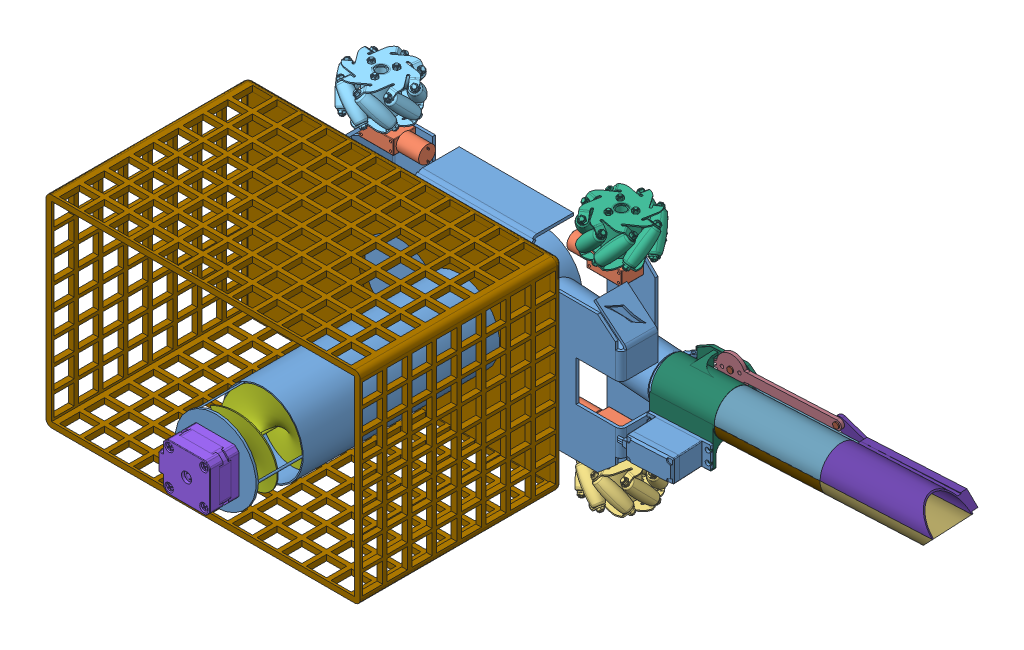
SolidWorks assembly tennis_car4, configuration 默认. Lengths in mm.
Overall size (577.55 226.09 334.13).
29 component instances, 19 part files, 66 mates.
Components (placement in the parent):
- car_main_body-1: car_main_body [默认] at (-145.051 -370.0736 71.4729) x (0 1 0) z (0 0 1) size (155.3 282.12 292.07)
- DC-1: DC [默认] at (85.5314 -436.576 -92.4792) x (-1 0 0) z (0 -1 0) size (53.09 20 29.75)
- Mecanum_wheel_RF-1: Mecanum_wheel_RF [默认] at (115.9795 -500.576 -23.0536) x (0 1 0) z (-0.527874 0 -0.849323) size (37 59.47 59.47)
- DC-2: DC [默认] at (-98.7631 -436.5721 -92.4792) x (1 0 0) z (0 -1 0) size (53.09 20 29.75)
- Mecanum_wheel_RB2-1: Mecanum_wheel_RB2 [默认] at (-98.0143 -496.5968 -67.0588) x (0 -1 0) z (-0.547075 0 -0.837084) size (37 61.04 61.04)
- DC-3: DC [默认] at (-98.7631 -344.5751 -92.4792) x (1 0 0) z (0 1 0) size (53.09 20 29.75)
- Mecanum_wheel_LB2-1: Mecanum_wheel_LB2 [默认] at (-99.6676 -280.5751 -22.7664) x (0 -1 0) z (0.13721 0 -0.990542) size (37 59.47 59.47)
- DC-4: DC [默认] at (85.5314 -344.5712 -92.4792) x (-1 0 0) z (0 1 0) size (53.09 20 29.75)
- Mecanum_wheel_LF2-1: Mecanum_wheel_LF2 [默认] at (125.629 -307.5959 -108.7375) x (0 -1 0) z (-0.82588 0 0.563846) size (37 61.04 61.04)
- spiral_tube-1: spiral_tube [默认] at (4.7184 -390.5736 -116.766) x (0.909362 0.416006 0) z (0 0 1) size (68 68 282.11)
- Stepper Motor3-1: Stepper Motor3 [默认] at (4.7184 -390.5736 198.234) x (0 1 0) z (-1 0 0) size (42 43 47.1)
- box2-1: box2 [默认] at (-48.4877 -300.5736 41.234) x (1 0 0) z (0 -1 0) size (280 180 180)
- part8-8-3: part8-8 [Default] at (159.2089 -414.9542 -121.0328) x (0.049403 0 0.998779) z (0.822654 -0.567084 -0.040691) size (30 17.5 17.5)
- Part6-6-17: Part6-6 [Default] at (266.8876 -408.5259 -124.3565) x (0.382581 -0.923728 -0.018924) z (-0.9226 -0.383049 0.045635) size (5 8 5)
- Part1-2-3: Part1-2 [Default] at (267.0852 -408.5259 -120.3614) x (0.926104 0.374476 -0.045808) z (-0.049403 0 -0.998779) size (119.31 46.68 44)
- Part6-6-18: Part6-6 [Default] at (266.9977 -377.0736 -124.3619) x (-0.382581 0.923728 0.018924) z (0.9226 0.383049 -0.045635) size (5 8 5)
- Part6-6-19: Part6-6 [Default] at (177.1076 -377.0736 -119.9157) x (-0.026872 -0.999638 0.001329) z (-0.998417 0.026905 0.049385) size (5 8 5)
- part5-5-3: part5-5 [Default] at (177.4534 -377.0736 -112.9243) x (-0.049403 0 -0.998779) z (-0.990234 -0.130526 0.04898) size (3 27.84 107.77)
- Part6-6-20: Part6-6 [Default] at (177.5028 -404.0736 -111.9255) x (-0.118763 -0.992905 0.005874) z (0.991693 -0.118909 -0.049052) size (5 8 5)
- Part2-2-3: Part2-2 [Default] at (197.7547 -385.3338 -115.4303) x (0.998779 0.000271 -0.049403) z (0.049403 0 0.998779) size (97 19 41)
- Part3-3-3: Part3-3 [Default] at (139.6032 -390.5736 -117.0594) x (0 -1 0) z (0.049403 0 0.998779) size (57.15 60.42 44.03)
- Part6-6-21: Part6-6 [Default] at (197.483 -385.3338 -120.9235) x (0.382581 -0.923728 -0.018924) z (-0.9226 -0.383049 0.045635) size (5 8 5)
- Part6-6-22: Part6-6 [Default] at (287.3731 -385.3094 -125.3698) x (0.382581 -0.923728 -0.018924) z (-0.9226 -0.383049 0.045635) size (5 8 5)
- Part6-6-23: Part6-6 [Default] at (287.2619 -400.2875 -125.3643) x (0.223935 -0.974541 -0.011077) z (-0.973351 -0.224209 0.048145) size (5 8 5)
- Part6-6-24: Part6-6 [Default] at (197.483 -395.8134 -120.9235) x (0.382581 -0.923728 -0.018924) z (-0.9226 -0.383049 0.045635) size (5 8 5)
- part4-4-3: part4-4 [Default] at (177.3052 -404.0736 -115.9206) x (0.049403 0 0.998779) z (-0.997556 0.049471 0.049342) size (3 29.07 108.54)
- Part1-1-3: Part1-1 [Default] at (267.0471 -377.0736 -123.3632) x (0.926153 -0.374355 -0.04581) z (0.049403 0 0.998779) size (117.54 46.76 44)
- Part2-1-3: Part2-1 [Default] at (287.5336 -400.2875 -119.871) x (-0.997544 0.049712 0.049342) z (0.049403 0 0.998779) size (97 23.44 41)
- 舵机-1: 舵机 [默认] at (171.737 -414.9542 -72.1921) x (-0.998779 0 0.049403) z (0 -1 0) size (56.95 44.55 19.71)
Mates (geometry in assembly coordinates):
- 同心1: concentric aligned: cylinder of car_main_body-1 through (4.7184 -390.5736 171.234) axis (0 0 -1) radius 36; cylinder of spiral_tube-1 through (4.7184 -390.5736 165.234) axis (0 0 -1) radius 1
- 重合13: coincident anti-aligned: plane of car_main_body-1 through (4.7184 -390.5736 -116.766) normal (0 0 1); plane of spiral_tube-1 through (4.7184 -390.5736 -116.766) normal (0 0 -1)
- 同心2: concentric aligned: cylinder of car_main_body-1 through (4.7184 -390.5736 171.234) axis (0 0 1) radius 11; cylinder of Stepper Motor3-1 through (4.7184 -390.5736 155.234) axis (0 0 1) radius 2.5
- 同心3: concentric aligned: circle of car_main_body-1; cone of Stepper Motor3-1 through (20.2184 -375.0736 173.234) axis (0 0 1)
- 重合16: coincident anti-aligned: plane of car_main_body-1 through (4.7184 -390.5736 173.234) normal (0 0 1); plane of Stepper Motor3-1 through (4.7184 -390.5736 173.234) normal (0 0 -1)
- 重合17: coincident anti-aligned: plane of car_main_body-1 through (4.7184 -390.5736 -48.766) normal (0 0 1); plane of box2-1 through (-188.4877 -480.5736 -48.766) normal (0 0 -1)
- 重合18: coincident aligned: plane of car_main_body-1 through (-145.051 -390.5736 71.4729) normal (0 -1 0); plane of box2-1 through (-48.4877 -390.5736 41.234) normal (0 -1 0)
- 同心35: concentric anti-aligned: cylinder of DC-1 through (100.5314 -477.576 -92.4792) axis (0 1 0) radius 4; cylinder of Mecanum_wheel_RF-1 through (100.5314 -470.576 -92.4792) axis (0 -1 0) radius 4
- 重合35: coincident anti-aligned: plane of DC-1 through (100.5314 -470.576 -92.4792) normal (0 -1 0); plane of Mecanum_wheel_RF-1 through (100.5314 -470.576 -92.4792) normal (0 1 0)
- 重合36: coincident: plane of DC-1 through (110.5314 -436.576 -102.4792) normal (0 0 -1); plane of car_main_body-1 through (100.4806 -390.5736 -102.4792) normal (0 0 1)
- 重合37: coincident: plane of car_main_body-1 through (-145.051 -461.576 71.4729) normal (0 -1 0); plane of DC-1 through (85.5314 -461.576 -92.4792) normal (0 -1 0)
- 重合38: coincident: line of car_main_body-1 through (110.5314 -461.576 -104.9792) axis (0 0 1); plane of DC-1 through (110.5314 -461.576 -107.4792) normal (1 0 0)
- 重合39: coincident: plane of car_main_body-1 through (-91.0439 -390.5736 -102.4792) normal (0 0 1); plane of DC-2 through (-123.7631 -436.5721 -102.4792) normal (0 0 -1)
- 重合40: coincident: plane of car_main_body-1 through (-123.6589 -461.5721 -103.9928) normal (0 -1 0); plane of DC-2 through (-98.7631 -461.5721 -92.4792) normal (0 -1 0)
- 重合41: coincident: line of car_main_body-1 through (-123.7631 -445.1021 -102.4792) axis (0 -1 0); plane of DC-2 through (-123.7631 -461.5721 -77.4792) normal (-1 0 0)
- 同心37: concentric anti-aligned: cylinder of DC-3 through (-113.7631 -303.5751 -92.4792) axis (0 -1 0) radius 4; cylinder of Mecanum_wheel_LB2-1 through (-113.7631 -310.5751 -92.4792) axis (0 1 0) radius 4
- 重合42: coincident anti-aligned: plane of DC-3 through (-113.7631 -310.5751 -92.4792) normal (0 1 0); plane of Mecanum_wheel_LB2-1 through (-113.7631 -310.5751 -92.4792) normal (0 -1 0)
- 重合43: coincident: plane of car_main_body-1 through (-91.0439 -390.5736 -102.4792) normal (0 0 1); plane of DC-3 through (-123.7631 -344.5751 -102.4792) normal (0 0 -1)
- 重合44: coincident: plane of car_main_body-1 through (-125.6782 -319.5751 -101.5862) normal (0 1 0); plane of DC-3 through (-98.7631 -319.5751 -92.4792) normal (0 1 0)
- 重合45: coincident: line of car_main_body-1 through (-123.7631 -319.5751 -102.4792) axis (0 -1 0); plane of DC-3 through (-123.7631 -319.5751 -107.4792) normal (-1 0 0)
- 重合47: coincident: plane of car_main_body-1 through (100.4806 -390.5736 -102.4792) normal (0 0 1); plane of DC-4 through (110.5314 -344.5712 -102.4792) normal (0 0 -1)
- 重合48: coincident: plane of car_main_body-1 through (-145.051 -319.5712 71.4729) normal (0 1 0); plane of DC-4 through (85.5314 -319.5712 -92.4792) normal (0 1 0)
- 重合49: coincident: line of car_main_body-1 through (110.5314 -319.5712 -102.4792) axis (0 0 -1); plane of DC-4 through (110.5314 -319.5712 -77.4792) normal (1 0 0)
- GearMate2: gear = 13 : 24 mm: cylinder of part8-8-3 through (159.7029 -414.9542 -111.045) axis (-0.049403 0 -0.998779) radius 5.249; cylinder of part4-4-3 through (177.4534 -404.0736 -112.9243) axis (-0.049403 0 -0.998779) radius 12.0927
- 重合20: coincident aligned: plane of Part3-3-3 through (139.6032 -390.5736 -117.0594) normal (-0.049403 0 -0.998779); plane of part8-8-3 through (159.3571 -414.9542 -118.0365) normal (-0.049403 0 -0.998779)
- 同心34: concentric anti-aligned: cylinder of Part3-3-3 through (157.6803 -414.9542 -151.9362) axis (0.049403 0 0.998779) radius 8.5; cylinder of part8-8-3 through (161.679 -414.9542 -71.0938) axis (-0.049403 0 -0.998779) radius 0.4
- Concentric24: concentric aligned: cylinder of part4-4-3 through (267.2334 -408.5259 -117.3651) axis (-0.049403 0 -0.998779) radius 1.5; cylinder of Part6-6-17 through (266.8876 -408.5259 -124.3565) axis (-0.049403 0 -0.998779) radius 1.5
- Coincident23: coincident anti-aligned: plane of part4-4-3 through (177.4534 -404.0736 -112.9243) normal (0.049403 0 0.998779); plane of Part6-6-17 through (266.277 -406.2166 -117.3177) normal (-0.049403 0 -0.998779)
- 平行6: parallel anti-aligned: cylinder of Part6-6-17 through (266.8876 -408.5259 -124.3565) axis (-0.049403 0 -0.998779) radius 2.5; cylinder of Part1-2-3 through (266.937 -408.5259 -123.3577) axis (0.049403 0 0.998779) radius 1.5
- 同心25: concentric anti-aligned: cylinder of Part6-6-17 through (266.8876 -408.5259 -124.3565) axis (-0.049403 0 -0.998779) radius 2.5; cylinder of Part1-2-3 through (266.937 -408.5259 -123.3577) axis (0.049403 0 0.998779) radius 1.5
- 重合56: coincident aligned: plane of Part1-1-3 through (267.1953 -377.0736 -120.3668) normal (0.049403 0 0.998779); plane of Part1-2-3 through (267.0852 -408.5259 -120.3614) normal (0.049403 0 0.998779)
- 同心26: concentric anti-aligned: cylinder of Part6-6-23 through (287.2619 -400.2875 -125.3643) axis (-0.049403 0 -0.998779) radius 2.5; cylinder of Part1-2-3 through (287.3113 -400.2875 -124.3655) axis (0.049403 0 0.998779) radius 1.5
- Concentric19: concentric anti-aligned: cylinder of part5-5-3 through (267.1953 -377.0736 -120.3668) axis (0.049403 0 0.998779) radius 1.5; cylinder of Part6-6-18 through (266.9977 -377.0736 -124.3619) axis (-0.049403 0 -0.998779) radius 1.5
- Coincident18: coincident anti-aligned: plane of part5-5-3 through (177.4534 -377.0736 -112.9243) normal (0.049403 0 0.998779); plane of Part6-6-18 through (268.3 -379.3829 -117.4178) normal (-0.049403 0 -0.998779)
- Concentric18: concentric anti-aligned: cylinder of part5-5-3 through (174.9833 -377.0736 -162.8633) axis (0.049403 0 0.998779) radius 1.5; cylinder of Part6-6-19 through (177.1076 -377.0736 -119.9157) axis (-0.049403 0 -0.998779) radius 1.5
- Coincident17: coincident anti-aligned: plane of part5-5-3 through (177.4534 -377.0736 -112.9243) normal (0.049403 0 0.998779); plane of Part6-6-19 through (177.5206 -374.5745 -112.9276) normal (-0.049403 0 -0.998779)
- Concentric2: concentric anti-aligned: cylinder of Part3-3-3 through (177.3052 -377.0736 -115.9206) axis (-0.049403 0 -0.998779) radius 1.5; cylinder of part5-5-3 through (174.9833 -377.0736 -162.8633) axis (0.049403 0 0.998779) radius 1.5
- Coincident3: coincident anti-aligned: plane of Part3-3-3 through (139.7514 -390.5736 -114.0631) normal (0.049403 0 0.998779); plane of part5-5-3 through (177.3052 -377.0736 -115.9206) normal (-0.049403 0 -0.998779)
- Concentric4: concentric anti-aligned: cylinder of part5-5-3 through (267.1953 -377.0736 -120.3668) axis (0.049403 0 0.998779) radius 1.5; cylinder of Part1-1-3 through (267.1953 -377.0736 -120.3668) axis (-0.049403 0 -0.998779) radius 1.5
- Coincident9: coincident anti-aligned: plane of part5-5-3 through (177.3052 -377.0736 -115.9206) normal (-0.049403 0 -0.998779); plane of Part1-1-3 through (267.1953 -377.0736 -120.3668) normal (0.049403 0 0.998779)
- LimitAngle1: limit planar angle = 3.141593 rad anti-aligned: plane of part5-5-3 through (177.3052 -373.0736 -115.9206) normal (0 1 0); plane of Part3-3-3 through (187.5926 -370.0736 -116.4294) normal (0 1 0)
- GearMate1: gear = 1 : 1 mm: cylinder of part5-5-3 through (177.3052 -377.0736 -115.9206) axis (0.049403 0 0.998779) radius 12.0927; cylinder of part4-4-3 through (177.4534 -404.0736 -112.9243) axis (-0.049403 0 -0.998779) radius 12.0927
- Concentric15: concentric anti-aligned: cylinder of part4-4-3 through (179.7753 -404.0736 -65.9816) axis (-0.049403 0 -0.998779) radius 1.5; cylinder of Part6-6-20 through (177.5028 -404.0736 -111.9255) axis (0.049403 0 0.998779) radius 1.5
- 重合61: coincident anti-aligned: plane of Part3-3-3 through (139.6032 -390.5736 -117.0594) normal (-0.049403 0 -0.998779); plane of Part6-6-20 through (177.4539 -401.5913 -118.9316) normal (0.049403 0 0.998779)
- Concentric3: concentric aligned: cylinder of Part3-3-3 through (197.6806 -385.3338 -116.9284) axis (-0.049403 0 -0.998779) radius 1.5; cylinder of Part2-2-3 through (197.8288 -385.3338 -113.9321) axis (-0.049403 0 -0.998779) radius 1.5
- Coincident4: coincident anti-aligned: plane of Part3-3-3 through (139.7514 -390.5736 -114.0631) normal (0.049403 0 0.998779); plane of Part2-2-3 through (197.6806 -385.3338 -116.9284) normal (-0.049403 0 -0.998779)
- Concentric20: concentric aligned: cylinder of Part2-2-3 through (197.8288 -385.3338 -113.9321) axis (-0.049403 0 -0.998779) radius 1.5; cylinder of Part6-6-21 through (197.483 -385.3338 -120.9235) axis (-0.049403 0 -0.998779) radius 1.5
- Coincident19: coincident anti-aligned: plane of Part2-2-3 through (197.8288 -385.3338 -113.9321) normal (0.049403 0 0.998779); plane of Part6-6-21 through (196.8723 -383.0244 -113.8848) normal (-0.049403 0 -0.998779)
- Concentric21: concentric aligned: cylinder of Part2-2-3 through (287.7189 -385.3094 -118.3783) axis (-0.049403 0 -0.998779) radius 1.5; cylinder of Part6-6-22 through (287.3731 -385.3094 -125.3698) axis (-0.049403 0 -0.998779) radius 1.5
- Coincident20: coincident anti-aligned: plane of Part2-2-3 through (197.8288 -385.3338 -113.9321) normal (0.049403 0 0.998779); plane of Part6-6-22 through (286.7624 -383.0001 -118.331) normal (-0.049403 0 -0.998779)
- Concentric1: concentric aligned: cylinder of Part3-3-3 through (177.3052 -404.0736 -115.9206) axis (-0.049403 0 -0.998779) radius 1.5; cylinder of part4-4-3 through (179.7753 -404.0736 -65.9816) axis (-0.049403 0 -0.998779) radius 1.5
- Coincident1: coincident anti-aligned: plane of Part3-3-3 through (139.7514 -390.5736 -114.0631) normal (0.049403 0 0.998779); plane of part4-4-3 through (177.3052 -404.0736 -115.9206) normal (-0.049403 0 -0.998779)
- 重合66: coincident anti-aligned: plane of Part3-3-3 through (139.7514 -390.5736 -114.0631) normal (0.049403 0 0.998779); plane of Part2-1-3 through (287.4595 -400.2875 -121.3692) normal (-0.049403 0 -0.998779)
- 同心33: concentric aligned: circle of Part3-3-3; cylinder of Part6-6-24 through (197.483 -395.8134 -120.9235) axis (-0.049403 0 -0.998779) radius 2.5
- 同心43: concentric aligned: cylinder of Part1-1-3 through (287.5707 -385.3094 -121.3747) axis (-0.049403 0 -0.998779) radius 1.5; cylinder of Part6-6-22 through (287.3731 -385.3094 -125.3698) axis (-0.049403 0 -0.998779) radius 2.5
- 同心27: concentric aligned: cylinder of Part6-6-23 through (287.2619 -400.2875 -125.3643) axis (-0.049403 0 -0.998779) radius 2.5; cylinder of Part2-1-3 through (287.6077 -400.2875 -118.3728) axis (-0.049403 0 -0.998779) radius 1.5
- 同心30: concentric aligned: cylinder of Part6-6-24 through (197.483 -395.8134 -120.9235) axis (-0.049403 0 -0.998779) radius 2.5; cylinder of Part2-1-3 through (197.8288 -395.8134 -113.9321) axis (-0.049403 0 -0.998779) radius 1.5
- 重合67: coincident: plane of assembly through (0 -390.5736 0) normal (0 1 0); plane of Part3-3-3 through (139.6032 -390.5736 -117.0594) normal (0 -1 0); plane of assembly
- 同心44: concentric: cylinder of car_main_body-1 through (143.8794 -400.5736 -113.266) axis (0 1 0) radius 1.5; cylinder of Part3-3-3 through (143.8794 -397.5736 -113.266) axis (0 1 0) radius 1.5
- 重合69: coincident anti-aligned: plane of DC-4 through (100.5314 -310.5712 -92.4792) normal (0 1 0); plane of Mecanum_wheel_LF2-1 through (100.5314 -310.5712 -92.4792) normal (0 -1 0)
- 同心47: concentric aligned: cylinder of DC-4 through (100.5314 -303.5712 -92.4792) axis (0 -1 0) radius 4; cylinder of Mecanum_wheel_LF2-1 through (100.5314 -281.5712 -92.4792) axis (0 -1 0) radius 4
- 重合71: coincident anti-aligned: plane of DC-2 through (-113.7631 -470.5721 -92.4792) normal (0 -1 0); plane of Mecanum_wheel_RB2-1 through (-113.7631 -470.5721 -92.4792) normal (0 1 0)
- 同心49: concentric anti-aligned: cylinder of DC-2 through (-113.7631 -477.5721 -92.4792) axis (0 1 0) radius 4; cylinder of Mecanum_wheel_RB2-1 through (-113.7631 -470.5721 -92.4792) axis (0 -1 0) radius 4
- 同心50: concentric aligned: cylinder of part8-8-3 through (159.8511 -414.9542 -108.0487) axis (-0.049403 0 -0.998779) radius 8.75; cylinder of 舵机-1 through (163.0474 -414.9542 -43.4277) axis (-0.049403 0 -0.998779) radius 1.2
- 平行7: parallel anti-aligned: plane of 舵机-1 through (171.737 -414.9542 -72.1921) normal (0 -1 0)
- 重合74: coincident anti-aligned: plane of Part3-3-3 through (144.6514 -370.0726 -73.2553) normal (0.049403 0 0.998779); plane of 舵机-1 through (198.3463 -408.4292 -75.9112) normal (-0.049403 0 -0.998779)
